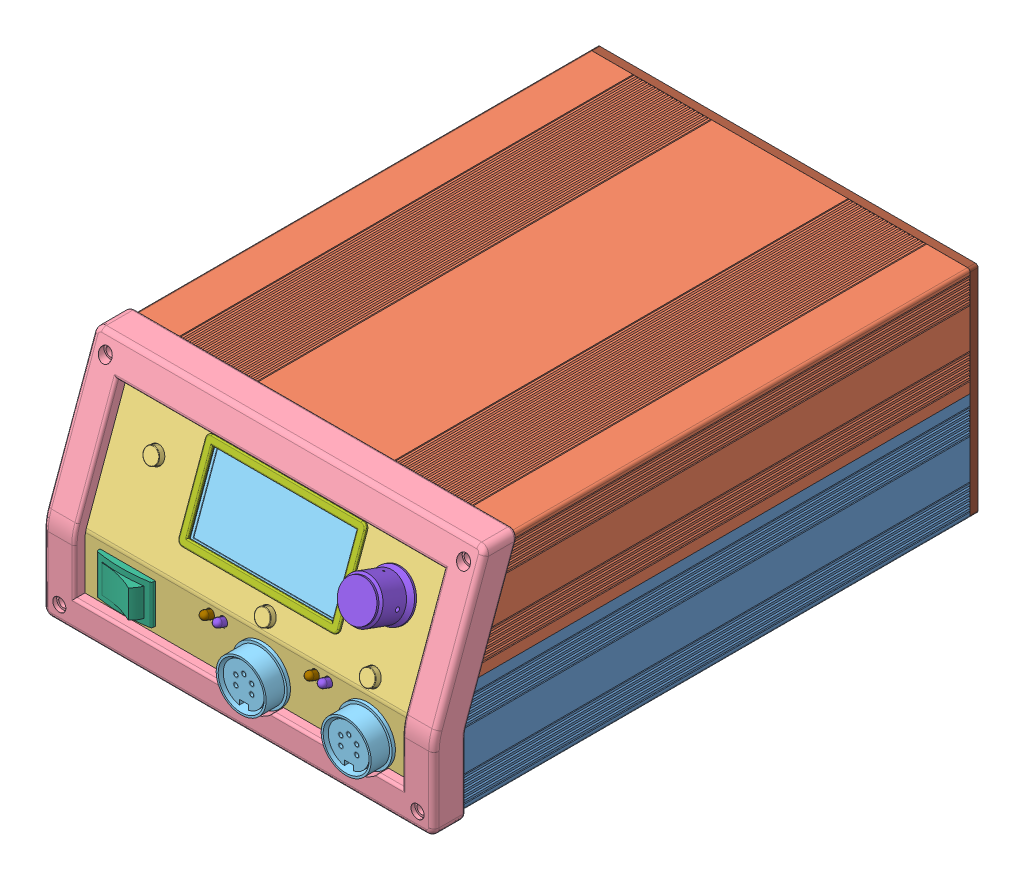
SolidWorks assembly Assembly, configuration Default. Lengths in mm.
Overall size (149 87.32 221.36).
420 component instances, 55 part files, 54 mates.
Components (placement in the parent):
- CaseExtrusion-ModifiedBottom-4: CaseExtrusion-ModifiedBottom [Default] at origin size (145 43.4 200)
- CaseExtrusion-ModifiedTop-7: CaseExtrusion-ModifiedTop [Default] x (-1 0 0) z (0 0 1) size (145 43.1 195.63)
- Front Panel-1: Front Panel [Default] at (72.5 -12 0) x (-1 0 0) z (0 0 -1) size (145 82.88 21.33)
- Front Panel Bezel-2: Front Panel Bezel [Default] at (0 -12 2.3103) x (0 0 1) z (-1 0 0) size (32.14 86.2 149)
- AmphenolSocket-3: AmphenolSocket [Default] at (5 -25.1 3.27) size (21 21 19.77)
- AmphenolSocket-4: AmphenolSocket [Default] at (45 -25.1 3.27) size (21 21 19.77)
- RockerSwitch-1: RockerSwitch [Default] at (-46.5075 -22.4992 2) x (-1 0 0) z (0 0 1) size (21.56 15.01 28.12)
- OledBezel-3: OledBezel [Default] at (0 14.2689 -6.3686) x (-1 0 0) z (0 -0.34202 -0.939693) size (61.1 33.49 3)
- Knob-1: Knob [HEA-A1-1] at (46 17.0964 -6.3335) x (1 0 0) z (0 -0.939693 0.34202) size (17.46 14.29 17.46)
- Transformer Mounting Plate-1: Transformer Mounting Plate [Default] at (0 -33.6 -100) size (115 2 115)
- Triad Magnetics-VPT48-3300-1: Triad Magnetics-VPT48-3300 [Default] at (0 -6.6 -100) x (0.526054 0 -0.850451) z (0.850451 0 0.526054) size (102.88 51 103.1)
- Rear Panel-1: Rear Panel [Default] at (0 0.01 -200) x (0 0 -1) z (1 0 0) size (3 82.2 145)
- IEC_Connector_Fused_Flanges (Schurter 6200)-1: IEC_Connector_Fused_Flanges (Schurter 6200) [Default] at (-44.5 -14.19 -205.5) x (1 0 0) z (0 0 -1) size (44 34 28.25)
- SolderingStation-3: SolderingStation [Default] at (108 -45.1633 3.8854) x (-1 0 0) z (0 -0.34202 -0.939693) size (142.21 62 43.76)
  - SolderingStation.step-1: SolderingStation.step [Default] at origin size (142.21 62 43.76)
    - Board_ss.step-1: Board_ss.step [Default] at origin size (140 62 1.69)
      - Open CASCADE STEP translator 6.8 4.1.1.step-1: Open CASCADE STEP translator 6.8 4.1.1.step [Default] at (0 0 -1.6914) size (140 62 1.69)
    - C17_ss.step-1: C17_ss.step [Default] at origin size (1.25 2 0.78)
      - User_Library-0805_SMD_Capacitor.step-1: User_Library-0805_SMD_Capacitor.step [Default] at (110.8455 64.7701 0) x (0 1 0) z (1 0 0) size (2 0.78 1.25)
    - R45_ss.step-1: R45_ss.step [Default] at origin size (1.7 0.8 0.56)
      - User_Library-RES_1609-0603.step-1: User_Library-RES_1609-0603.step [Default] at (65.2781 57.15 0) x (1 0 0) z (0 -1 0) size (1.7 0.56 0.8)
    - N1_ss.step-1: N1_ss.step [Default] at origin size (9.09 12.8 3.73)
      - nal-clip.step-1: nal-clip.step [Default] at (42.9877 48.2091 -0.8) x (0 0 -1) z (0 -1 0) size (3.73 9.09 12.8)
    - U2_ss.step-1: U2_ss.step [Default] at origin size (6.2 5 1.75)
      - User_Library-SOIC8_JEDEC_MS-012AA.step-1: User_Library-SOIC8_JEDEC_MS-012AA.step [Default] at (80.8676 75.6667 0) x (0 1 0) z (1 0 0) size (5 1.75 6.2)
    - C15_ss.step-1: C15_ss.step [Default] at origin size (1.6 0.8 0.3)
      - User_Library-0603_SMD_Capacitor.step-1: User_Library-0603_SMD_Capacitor.step [Default] at (161.9249 74.0409 0) x (-1 0 0) z (0 1 0) size (1.6 0.3 0.8)
    - C18_ss.step-1: C18_ss.step [Default] at origin size (1.6 0.8 0.3)
      - User_Library-0603_SMD_Capacitor.step-1: User_Library-0603_SMD_Capacitor.step [Default] at (161.9249 75.4379 0) x (-1 0 0) z (0 1 0) size (1.6 0.3 0.8)
    - U10_ss.step-1: U10_ss.step [Default] at origin size (3 2.5 1.1)
      - CircuitWorks-SOT-23.step-1: CircuitWorks-SOT-23.step [Default] at (163.4489 78.7147 0.5) x (-1 0 0) z (0 1 0) size (3 1.1 2.5)
    - U9_ss.step-1: U9_ss.step [Default] at origin size (2.8 2.9 1.45)
      - User_Library-SOT23-5-2.step-1: User_Library-SOT23-5-2.step [Default] at (107.9245 64.4143 0) x (0 -1 0) z (0 0 1) size (2.9 2.8 1.45)
    - C27_ss.step-1: C27_ss.step [Default] at origin size (1.25 2 0.78)
      - User_Library-0805_SMD_Capacitor.step-1: User_Library-0805_SMD_Capacitor.step [Default] at (114.5539 60.8331 0) x (0 1 0) z (1 0 0) size (2 0.78 1.25)
    - C26_ss.step-1: C26_ss.step [Default] at origin size (0.8 1.6 0.3)
      - User_Library-0603_SMD_Capacitor.step-1: User_Library-0603_SMD_Capacitor.step [Default] at (105.0035 64.1605 0) x (0 1 0) z (1 0 0) size (1.6 0.3 0.8)
    - C25_ss.step-1: C25_ss.step [Default] at origin size (1.25 2 0.78)
      - User_Library-0805_SMD_Capacitor.step-1: User_Library-0805_SMD_Capacitor.step [Default] at (109.4741 44.7039 0) x (0 -1 0) z (-1 0 0) size (2 0.78 1.25)
    - C24_ss.step-1: C24_ss.step [Default] at origin size (1.25 2 0.78)
      - User_Library-0805_SMD_Capacitor.step-1: User_Library-0805_SMD_Capacitor.step [Default] at (69.5961 44.4499 0) x (0 -1 0) z (-1 0 0) size (2 0.78 1.25)
    - D13_ss.step-1: D13_ss.step [Default] at origin size (2.7 1.25 1.1)
      - User_Library-SOD2513X11.step-1: User_Library-SOD2513X11.step [Default] at (167.7671 78.5115 0) x (1 0 0) z (0 0 1) size (2.7 1.25 1.1)
    - C22_ss.step-1: C22_ss.step [Default] at origin size (2 1.25 0.78)
      - User_Library-0805_SMD_Capacitor.step-1: User_Library-0805_SMD_Capacitor.step [Default] at (105.3871 57.6581 0) x (1 0 0) z (0 -1 0) size (2 0.78 1.25)
    - C23_ss.step-1: C23_ss.step [Default] at origin size (2 1.25 0.78)
      - User_Library-0805_SMD_Capacitor.step-1: User_Library-0805_SMD_Capacitor.step [Default] at (111.2291 57.6581 0) x (1 0 0) z (0 -1 0) size (2 0.78 1.25)
    - C21_ss.step-1: C21_ss.step [Default] at origin size (1.6 0.8 0.3)
      - User_Library-0603_SMD_Capacitor.step-1: User_Library-0603_SMD_Capacitor.step [Default] at (102.3367 85.0901 0) x (1 0 0) z (0 -1 0) size (1.6 0.3 0.8)
    - SP6_ss.step-1: SP6_ss.step [Default] at origin size (6 6 6)
      - 6mmSpacer.step-1: 6mmSpacer.step [Default] at (46.8629 36.8301 -1.6914) x (-1 0 0) z (0 -1 0) size (6 6 6)
    - SP5_ss.step-1: SP5_ss.step [Default] at origin size (6 6 6)
      - 6mmSpacer.step-1: 6mmSpacer.step [Default] at (169.9259 46.8631 -1.6914) x (-1 0 0) z (0 -1 0) size (6 6 6)
    - D2_ss.step-1: D2_ss.step [Default] at origin size (2.7 1.25 1.1)
      - User_Library-SOD2513X11.step-1: User_Library-SOD2513X11.step [Default] at (125.2719 47.6779 0) x (-1 0 0) z (0 0 1) size (2.7 1.25 1.1)
    - U1_ss.step-1: U1_ss.step [Default] at origin size (9.94 6.54 2.42)
      - User_Library-DPAK-1.step-1: User_Library-DPAK-1.step [Default] at (105.596 76.2 1.15) x (0 -1 0) z (-1 0 0) size (6.54 2.42 9.94)
    - C20_ss.step-1: C20_ss.step [Default] at origin size (0.8 1.6 0.3)
      - User_Library-0603_SMD_Capacitor.step-1: User_Library-0603_SMD_Capacitor.step [Default] at (132.4355 61.1887 0) x (0 1 0) z (1 0 0) size (1.6 0.3 0.8)
    - C7_ss.step-1: C7_ss.step [Default] at origin size (0.8 1.6 0.3)
      - User_Library-0603_SMD_Capacitor.step-1: User_Library-0603_SMD_Capacitor.step [Default] at (92.3797 61.1631 0) x (0 1 0) z (1 0 0) size (1.6 0.3 0.8)
    - P1_ss.step-1: P1_ss.step [Default] at origin size (10.62 6.5 13.4)
      - c-282834-4-c-3d.step-1: c-282834-4-c-3d.step [Default] at (138.4201 36.0681 10) size (10.62 6.5 13.4)
    - R25_ss.step-1: R25_ss.step [Default] at origin size (1.65 16.48 27.41)
      - OAR3.step-1: OAR3.step [Default] at (70.9931 46.1009 -3.2) x (0 -1 0) z (-1 0 0) size (16.48 27.41 1.65)
    - R26_ss.step-1: R26_ss.step [Default] at origin size (1.65 16.48 27.41)
      - OAR3.step-1: OAR3.step [Default] at (111.1505 46.1009 -3.2) x (0 -1 0) z (-1 0 0) size (16.48 27.41 1.65)
    - R19_ss.step-1: R19_ss.step [Default] at origin size (0.8 1.7 0.56)
      - User_Library-RES_1609-0603.step-1: User_Library-RES_1609-0603.step [Default] at (154.101 48.0431 0) x (0 1 0) z (1 0 0) size (1.7 0.56 0.8)
    - R20_ss.step-1: R20_ss.step [Default] at origin size (0.8 1.7 0.56)
      - User_Library-RES_1609-0603.step-1: User_Library-RES_1609-0603.step [Default] at (156.1329 48.0431 0) x (0 1 0) z (1 0 0) size (1.7 0.56 0.8)
    - R27_ss.step-1: R27_ss.step [Default] at origin size (0.8 1.7 0.56)
      - User_Library-RES_1609-0603.step-1: User_Library-RES_1609-0603.step [Default] at (154.101 40.5501 0) x (0 1 0) z (1 0 0) size (1.7 0.56 0.8)
    - R28_ss.step-1: R28_ss.step [Default] at origin size (0.8 1.7 0.56)
      - User_Library-RES_1609-0603.step-1: User_Library-RES_1609-0603.step [Default] at (156.1329 40.5501 0) x (0 1 0) z (1 0 0) size (1.7 0.56 0.8)
    - D11_ss.step-1: D11_ss.step [Default] at origin size (3.5 3.8 10)
      - Red-LED_3MM.step-1: Red-LED_3MM.step [Default] at (77.9999 28.5001 -5.6914) x (0 1 0) z (0 0 -1) size (3.8 3.5 10)
    - D9_ss.step-1: D9_ss.step [Default] at origin size (3.5 3.8 10)
      - Red-LED_3MM.step-1: Red-LED_3MM.step [Default] at (117.9999 28.5001 -5.6914) x (0 1 0) z (0 0 -1) size (3.8 3.5 10)
    - D10_ss.step-1: D10_ss.step [Default] at origin size (3.5 3.8 10)
      - Green-LED_3MM.step-1: Green-LED_3MM.step [Default] at (122.9999 28.5001 -5.6914) x (0 1 0) z (0 0 -1) size (3.8 3.5 10)
    - D12_ss.step-1: D12_ss.step [Default] at origin size (3.5 3.8 10)
      - Green-LED_3MM.step-1: Green-LED_3MM.step [Default] at (82.9999 28.5001 -5.6914) x (0 1 0) z (0 0 -1) size (3.8 3.5 10)
    - S2_ss.step-1: S2_ss.step [Default] at origin size (7.7 6 10.2)
      - User_Library-b3w1050.step-1: User_Library-b3w1050.step [Default] at (63 36.9999 -1.6914) x (1 0 0) z (0 1 0) size (3.5 1.6 3.5)
      - User_Library-b3w1050.step-2: User_Library-b3w1050.step [Default] at (63 36.9999 -1.6914) x (1 0 0) z (0 1 0) size (3.5 1.6 3.5)
      - User_Library-b3w1050-0.step-1: User_Library-b3w1050-0.step [Default] at (63 36.9999 -1.6914) x (1 0 0) z (0 1 0) size (3.5 1.6 3.5)
      - User_Library-b3w1050-1.step-1: User_Library-b3w1050-1.step [Default] at (63 36.9999 -1.6914) x (1 0 0) z (0 1 0) size (7.7 10.2 6)
      - User_Library-b3w1050-1.step-2: User_Library-b3w1050-1.step [Default] at (63 36.9999 -1.6914) x (1 0 0) z (0 1 0) size (7.7 10.2 6)
      - User_Library-b3w1050-2.step-1: User_Library-b3w1050-2.step [Default] at (63 36.9999 -1.6914) x (1 0 0) z (0 1 0) size (7.7 10.2 6)
    - S1_ss.step-1: S1_ss.step [Default] at origin size (7.7 6 10.2)
      - User_Library-b3w1050.step-1: User_Library-b3w1050.step [Default] at (154 62.0001 -1.6914) x (-1 0 0) z (0 -1 0) size (3.5 1.6 3.5)
      - User_Library-b3w1050.step-2: User_Library-b3w1050.step [Default] at (154 62.0001 -1.6914) x (-1 0 0) z (0 -1 0) size (3.5 1.6 3.5)
      - User_Library-b3w1050-0.step-1: User_Library-b3w1050-0.step [Default] at (154 62.0001 -1.6914) x (-1 0 0) z (0 -1 0) size (3.5 1.6 3.5)
      - User_Library-b3w1050-1.step-1: User_Library-b3w1050-1.step [Default] at (154 62.0001 -1.6914) x (-1 0 0) z (0 -1 0) size (7.7 10.2 6)
      - User_Library-b3w1050-1.step-2: User_Library-b3w1050-1.step [Default] at (154 62.0001 -1.6914) x (-1 0 0) z (0 -1 0) size (7.7 10.2 6)
      - User_Library-b3w1050-2.step-1: User_Library-b3w1050-2.step [Default] at (154 62.0001 -1.6914) x (-1 0 0) z (0 -1 0) size (7.7 10.2 6)
    - S3_ss.step-1: S3_ss.step [Default] at origin size (7.7 6 10.2)
      - User_Library-b3w1050.step-1: User_Library-b3w1050.step [Default] at (103 36.9999 -1.6914) x (1 0 0) z (0 1 0) size (3.5 1.6 3.5)
      - User_Library-b3w1050.step-2: User_Library-b3w1050.step [Default] at (103 36.9999 -1.6914) x (1 0 0) z (0 1 0) size (3.5 1.6 3.5)
      - User_Library-b3w1050-0.step-1: User_Library-b3w1050-0.step [Default] at (103 36.9999 -1.6914) x (1 0 0) z (0 1 0) size (3.5 1.6 3.5)
      - User_Library-b3w1050-1.step-1: User_Library-b3w1050-1.step [Default] at (103 36.9999 -1.6914) x (1 0 0) z (0 1 0) size (7.7 10.2 6)
      - User_Library-b3w1050-1.step-2: User_Library-b3w1050-1.step [Default] at (103 36.9999 -1.6914) x (1 0 0) z (0 1 0) size (7.7 10.2 6)
      - User_Library-b3w1050-2.step-1: User_Library-b3w1050-2.step [Default] at (103 36.9999 -1.6914) x (1 0 0) z (0 1 0) size (7.7 10.2 6)
    - U5_ss.step-1: U5_ss.step [Default] at origin size (9 9 1.6)
      - User_Library-LQFP48_Grid_0.5.step-1: User_Library-LQFP48_Grid_0.5.step [Default] at (153.5238 71.918 0) x (0 1 0) z (1 0 0) size (9 1.6 9)
        - User_Library-LQFP48_Grid_0.5_LQFP48_Koerper_2.step-1: User_Library-LQFP48_Grid_0.5_LQFP48_Koerper_2.step [Default] at origin size (7 1.45 7)
        - User_Library-LQFP48_Grid_0.5_LQFP_PIN_2.step-1: User_Library-LQFP48_Grid_0.5_LQFP_PIN_2.step [Default] at (-2.75 0 4.5) size (0.27 0.97 1.5)
        - User_Library-LQFP48_Grid_0.5_LQFP_PIN_2.step-2: User_Library-LQFP48_Grid_0.5_LQFP_PIN_2.step [Default] at (-2.25 0 4.5) size (0.27 0.97 1.5)
        - User_Library-LQFP48_Grid_0.5_LQFP_PIN_2.step-3: User_Library-LQFP48_Grid_0.5_LQFP_PIN_2.step [Default] at (-1.75 0 4.5) size (0.27 0.97 1.5)
        - User_Library-LQFP48_Grid_0.5_LQFP_PIN_2.step-4: User_Library-LQFP48_Grid_0.5_LQFP_PIN_2.step [Default] at (-1.25 0 4.5) size (0.27 0.97 1.5)
        - User_Library-LQFP48_Grid_0.5_LQFP_PIN_2.step-5: User_Library-LQFP48_Grid_0.5_LQFP_PIN_2.step [Default] at (-0.75 0 4.5) size (0.27 0.97 1.5)
        - User_Library-LQFP48_Grid_0.5_LQFP_PIN_2.step-6: User_Library-LQFP48_Grid_0.5_LQFP_PIN_2.step [Default] at (-0.25 0 4.5) size (0.27 0.97 1.5)
        - User_Library-LQFP48_Grid_0.5_LQFP_PIN_2.step-7: User_Library-LQFP48_Grid_0.5_LQFP_PIN_2.step [Default] at (0.25 0 4.5) size (0.27 0.97 1.5)
        - User_Library-LQFP48_Grid_0.5_LQFP_PIN_2.step-8: User_Library-LQFP48_Grid_0.5_LQFP_PIN_2.step [Default] at (0.75 0 4.5) size (0.27 0.97 1.5)
        - User_Library-LQFP48_Grid_0.5_LQFP_PIN_2.step-9: User_Library-LQFP48_Grid_0.5_LQFP_PIN_2.step [Default] at (1.25 0 4.5) size (0.27 0.97 1.5)
        - User_Library-LQFP48_Grid_0.5_LQFP_PIN_2.step-10: User_Library-LQFP48_Grid_0.5_LQFP_PIN_2.step [Default] at (1.75 0 4.5) size (0.27 0.97 1.5)
        - User_Library-LQFP48_Grid_0.5_LQFP_PIN_2.step-11: User_Library-LQFP48_Grid_0.5_LQFP_PIN_2.step [Default] at (2.25 0 4.5) size (0.27 0.97 1.5)
        - User_Library-LQFP48_Grid_0.5_LQFP_PIN_2.step-12: User_Library-LQFP48_Grid_0.5_LQFP_PIN_2.step [Default] at (2.75 0 4.5) size (0.27 0.97 1.5)
        - User_Library-LQFP48_Grid_0.5_LQFP_PIN_2.step-13: User_Library-LQFP48_Grid_0.5_LQFP_PIN_2.step [Default] at (4.5 0 2.75) x (0 0 -1) z (1 0 0) size (0.27 0.97 1.5)
        - User_Library-LQFP48_Grid_0.5_LQFP_PIN_2.step-14: User_Library-LQFP48_Grid_0.5_LQFP_PIN_2.step [Default] at (4.5 0 2.25) x (0 0 -1) z (1 0 0) size (0.27 0.97 1.5)
        - User_Library-LQFP48_Grid_0.5_LQFP_PIN_2.step-15: User_Library-LQFP48_Grid_0.5_LQFP_PIN_2.step [Default] at (4.5 0 1.75) x (0 0 -1) z (1 0 0) size (0.27 0.97 1.5)
        - User_Library-LQFP48_Grid_0.5_LQFP_PIN_2.step-16: User_Library-LQFP48_Grid_0.5_LQFP_PIN_2.step [Default] at (4.5 0 1.25) x (0 0 -1) z (1 0 0) size (0.27 0.97 1.5)
        - User_Library-LQFP48_Grid_0.5_LQFP_PIN_2.step-17: User_Library-LQFP48_Grid_0.5_LQFP_PIN_2.step [Default] at (4.5 0 0.75) x (0 0 -1) z (1 0 0) size (0.27 0.97 1.5)
        - User_Library-LQFP48_Grid_0.5_LQFP_PIN_2.step-18: User_Library-LQFP48_Grid_0.5_LQFP_PIN_2.step [Default] at (4.5 0 0.25) x (0 0 -1) z (1 0 0) size (0.27 0.97 1.5)
        - User_Library-LQFP48_Grid_0.5_LQFP_PIN_2.step-19: User_Library-LQFP48_Grid_0.5_LQFP_PIN_2.step [Default] at (4.5 0 -0.25) x (0 0 -1) z (1 0 0) size (0.27 0.97 1.5)
        - User_Library-LQFP48_Grid_0.5_LQFP_PIN_2.step-20: User_Library-LQFP48_Grid_0.5_LQFP_PIN_2.step [Default] at (4.5 0 -0.75) x (0 0 -1) z (1 0 0) size (0.27 0.97 1.5)
        - User_Library-LQFP48_Grid_0.5_LQFP_PIN_2.step-21: User_Library-LQFP48_Grid_0.5_LQFP_PIN_2.step [Default] at (4.5 0 -1.25) x (0 0 -1) z (1 0 0) size (0.27 0.97 1.5)
        - User_Library-LQFP48_Grid_0.5_LQFP_PIN_2.step-22: User_Library-LQFP48_Grid_0.5_LQFP_PIN_2.step [Default] at (4.5 0 -1.75) x (0 0 -1) z (1 0 0) size (0.27 0.97 1.5)
        - User_Library-LQFP48_Grid_0.5_LQFP_PIN_2.step-23: User_Library-LQFP48_Grid_0.5_LQFP_PIN_2.step [Default] at (4.5 0 -2.25) x (0 0 -1) z (1 0 0) size (0.27 0.97 1.5)
        - User_Library-LQFP48_Grid_0.5_LQFP_PIN_2.step-24: User_Library-LQFP48_Grid_0.5_LQFP_PIN_2.step [Default] at (4.5 0 -2.75) x (0 0 -1) z (1 0 0) size (0.27 0.97 1.5)
        - User_Library-LQFP48_Grid_0.5_LQFP_PIN_2.step-25: User_Library-LQFP48_Grid_0.5_LQFP_PIN_2.step [Default] at (2.75 0 -4.5) x (-1 0 0) z (0 0 -1) size (0.27 0.97 1.5)
        - User_Library-LQFP48_Grid_0.5_LQFP_PIN_2.step-26: User_Library-LQFP48_Grid_0.5_LQFP_PIN_2.step [Default] at (2.25 0 -4.5) x (-1 0 0) z (0 0 -1) size (0.27 0.97 1.5)
        - User_Library-LQFP48_Grid_0.5_LQFP_PIN_2.step-27: User_Library-LQFP48_Grid_0.5_LQFP_PIN_2.step [Default] at (1.75 0 -4.5) x (-1 0 0) z (0 0 -1) size (0.27 0.97 1.5)
        - User_Library-LQFP48_Grid_0.5_LQFP_PIN_2.step-28: User_Library-LQFP48_Grid_0.5_LQFP_PIN_2.step [Default] at (1.25 0 -4.5) x (-1 0 0) z (0 0 -1) size (0.27 0.97 1.5)
        - User_Library-LQFP48_Grid_0.5_LQFP_PIN_2.step-29: User_Library-LQFP48_Grid_0.5_LQFP_PIN_2.step [Default] at (0.75 0 -4.5) x (-1 0 0) z (0 0 -1) size (0.27 0.97 1.5)
        - User_Library-LQFP48_Grid_0.5_LQFP_PIN_2.step-30: User_Library-LQFP48_Grid_0.5_LQFP_PIN_2.step [Default] at (0.25 0 -4.5) x (-1 0 0) z (0 0 -1) size (0.27 0.97 1.5)
        - User_Library-LQFP48_Grid_0.5_LQFP_PIN_2.step-31: User_Library-LQFP48_Grid_0.5_LQFP_PIN_2.step [Default] at (-0.25 0 -4.5) x (-1 0 0) z (0 0 -1) size (0.27 0.97 1.5)
        - User_Library-LQFP48_Grid_0.5_LQFP_PIN_2.step-32: User_Library-LQFP48_Grid_0.5_LQFP_PIN_2.step [Default] at (-0.75 0 -4.5) x (-1 0 0) z (0 0 -1) size (0.27 0.97 1.5)
        - User_Library-LQFP48_Grid_0.5_LQFP_PIN_2.step-33: User_Library-LQFP48_Grid_0.5_LQFP_PIN_2.step [Default] at (-1.25 0 -4.5) x (-1 0 0) z (0 0 -1) size (0.27 0.97 1.5)
        - User_Library-LQFP48_Grid_0.5_LQFP_PIN_2.step-34: User_Library-LQFP48_Grid_0.5_LQFP_PIN_2.step [Default] at (-1.75 0 -4.5) x (-1 0 0) z (0 0 -1) size (0.27 0.97 1.5)
        - User_Library-LQFP48_Grid_0.5_LQFP_PIN_2.step-35: User_Library-LQFP48_Grid_0.5_LQFP_PIN_2.step [Default] at (-2.25 0 -4.5) x (-1 0 0) z (0 0 -1) size (0.27 0.97 1.5)
        - User_Library-LQFP48_Grid_0.5_LQFP_PIN_2.step-36: User_Library-LQFP48_Grid_0.5_LQFP_PIN_2.step [Default] at (-2.75 0 -4.5) x (-1 0 0) z (0 0 -1) size (0.27 0.97 1.5)
        - User_Library-LQFP48_Grid_0.5_LQFP_PIN_2.step-37: User_Library-LQFP48_Grid_0.5_LQFP_PIN_2.step [Default] at (-4.5 0 -2.75) x (0 0 1) z (-1 0 0) size (0.27 0.97 1.5)
        - User_Library-LQFP48_Grid_0.5_LQFP_PIN_2.step-38: User_Library-LQFP48_Grid_0.5_LQFP_PIN_2.step [Default] at (-4.5 0 -2.25) x (0 0 1) z (-1 0 0) size (0.27 0.97 1.5)
        - User_Library-LQFP48_Grid_0.5_LQFP_PIN_2.step-39: User_Library-LQFP48_Grid_0.5_LQFP_PIN_2.step [Default] at (-4.5 0 -1.75) x (0 0 1) z (-1 0 0) size (0.27 0.97 1.5)
        - User_Library-LQFP48_Grid_0.5_LQFP_PIN_2.step-40: User_Library-LQFP48_Grid_0.5_LQFP_PIN_2.step [Default] at (-4.5 0 -1.25) x (0 0 1) z (-1 0 0) size (0.27 0.97 1.5)
        - User_Library-LQFP48_Grid_0.5_LQFP_PIN_2.step-41: User_Library-LQFP48_Grid_0.5_LQFP_PIN_2.step [Default] at (-4.5 0 -0.75) x (0 0 1) z (-1 0 0) size (0.27 0.97 1.5)
        - User_Library-LQFP48_Grid_0.5_LQFP_PIN_2.step-42: User_Library-LQFP48_Grid_0.5_LQFP_PIN_2.step [Default] at (-4.5 0 -0.25) x (0 0 1) z (-1 0 0) size (0.27 0.97 1.5)
        - User_Library-LQFP48_Grid_0.5_LQFP_PIN_2.step-43: User_Library-LQFP48_Grid_0.5_LQFP_PIN_2.step [Default] at (-4.5 0 0.25) x (0 0 1) z (-1 0 0) size (0.27 0.97 1.5)
        - User_Library-LQFP48_Grid_0.5_LQFP_PIN_2.step-44: User_Library-LQFP48_Grid_0.5_LQFP_PIN_2.step [Default] at (-4.5 0 0.75) x (0 0 1) z (-1 0 0) size (0.27 0.97 1.5)
        - User_Library-LQFP48_Grid_0.5_LQFP_PIN_2.step-45: User_Library-LQFP48_Grid_0.5_LQFP_PIN_2.step [Default] at (-4.5 0 1.25) x (0 0 1) z (-1 0 0) size (0.27 0.97 1.5)
        - User_Library-LQFP48_Grid_0.5_LQFP_PIN_2.step-46: User_Library-LQFP48_Grid_0.5_LQFP_PIN_2.step [Default] at (-4.5 0 1.75) x (0 0 1) z (-1 0 0) size (0.27 0.97 1.5)
        - User_Library-LQFP48_Grid_0.5_LQFP_PIN_2.step-47: User_Library-LQFP48_Grid_0.5_LQFP_PIN_2.step [Default] at (-4.5 0 2.25) x (0 0 1) z (-1 0 0) size (0.27 0.97 1.5)
        - User_Library-LQFP48_Grid_0.5_LQFP_PIN_2.step-48: User_Library-LQFP48_Grid_0.5_LQFP_PIN_2.step [Default] at (-4.5 0 2.75) x (0 0 1) z (-1 0 0) size (0.27 0.97 1.5)
    - C12_ss.step-1: C12_ss.step [Default] at origin size (1.6 0.8 0.3)
      - User_Library-0603_SMD_Capacitor.step-1: User_Library-0603_SMD_Capacitor.step [Default] at (167.9195 75.9461 0) x (1 0 0) z (0 -1 0) size (1.6 0.3 0.8)
    - C13_ss.step-1: C13_ss.step [Default] at origin size (1.6 0.8 0.3)
      - User_Library-0603_SMD_Capacitor.step-1: User_Library-0603_SMD_Capacitor.step [Default] at (161.9249 72.1359 0) x (-1 0 0) z (0 1 0) size (1.6 0.3 0.8)
    - C14_ss.step-1: C14_ss.step [Default] at origin size (1.6 0.8 0.3)
      - User_Library-0603_SMD_Capacitor.step-1: User_Library-0603_SMD_Capacitor.step [Default] at (150.8761 78.6131 0) x (1 0 0) z (0 -1 0) size (1.6 0.3 0.8)
    - C16_ss.step-1: C16_ss.step [Default] at origin size (1.6 0.8 0.3)
      - User_Library-0603_SMD_Capacitor.step-1: User_Library-0603_SMD_Capacitor.step [Default] at (160.3239 66.9819 0) x (-1 0 0) z (0 1 0) size (1.6 0.3 0.8)
    - P6_ss.step-1: P6_ss.step [Default] at origin size (6.35 3.4 6.8)
      - SWD2x5.step-1: SWD2x5.step [Default] at (153.0859 83.8493 0) x (1 0 0) z (0 -1 0) size (6.35 6.8 3.4)
    - R38_ss.step-1: R38_ss.step [Default] at origin size (1.7 0.8 0.56)
      - User_Library-RES_1609-0603.step-1: User_Library-RES_1609-0603.step [Default] at (159.9431 62.537 0) x (1 0 0) z (0 -1 0) size (1.7 0.56 0.8)
    - R37_ss.step-1: R37_ss.step [Default] at origin size (1.7 0.8 0.56)
      - User_Library-RES_1609-0603.step-1: User_Library-RES_1609-0603.step [Default] at (159.9431 63.807 0) x (1 0 0) z (0 -1 0) size (1.7 0.56 0.8)
    - R40_ss.step-1: R40_ss.step [Default] at origin size (1.7 0.8 0.56)
      - User_Library-RES_1609-0603.step-1: User_Library-RES_1609-0603.step [Default] at (159.9431 61.267 0) x (1 0 0) z (0 -1 0) size (1.7 0.56 0.8)
    - R39_ss.step-1: R39_ss.step [Default] at origin size (1.7 0.8 0.56)
      - User_Library-RES_1609-0603.step-1: User_Library-RES_1609-0603.step [Default] at (172.3891 66.7281 0) x (1 0 0) z (0 -1 0) size (1.7 0.56 0.8)
    - R41_ss.step-1: R41_ss.step [Default] at origin size (1.7 0.8 0.56)
      - User_Library-RES_1609-0603.step-1: User_Library-RES_1609-0603.step [Default] at (172.3889 79.936 0) x (-1 0 0) z (0 1 0) size (1.7 0.56 0.8)
    - R42_ss.step-1: R42_ss.step [Default] at origin size (1.7 0.8 0.56)
      - User_Library-RES_1609-0603.step-1: User_Library-RES_1609-0603.step [Default] at (161.8479 70.5379 0) x (-1 0 0) z (0 1 0) size (1.7 0.56 0.8)
    - R43_ss.step-1: R43_ss.step [Default] at origin size (1.7 0.8 0.56)
      - User_Library-RES_1609-0603.step-1: User_Library-RES_1609-0603.step [Default] at (161.8479 69.268 0) x (-1 0 0) z (0 1 0) size (1.7 0.56 0.8)
    - R50_ss.step-1: R50_ss.step [Default] at origin size (1.7 0.8 0.56)
      - User_Library-RES_1609-0603.step-1: User_Library-RES_1609-0603.step [Default] at (77.5201 31.406 0) x (1 0 0) z (0 -1 0) size (1.7 0.56 0.8)
    - R47_ss.step-1: R47_ss.step [Default] at origin size (1.7 0.8 0.56)
      - User_Library-RES_1609-0603.step-1: User_Library-RES_1609-0603.step [Default] at (117.6519 31.422 0) x (-1 0 0) z (0 1 0) size (1.7 0.56 0.8)
    - R49_ss.step-1: R49_ss.step [Default] at origin size (1.7 0.8 0.56)
      - User_Library-RES_1609-0603.step-1: User_Library-RES_1609-0603.step [Default] at (122.7321 31.422 0) x (1 0 0) z (0 -1 0) size (1.7 0.56 0.8)
    - R52_ss.step-1: R52_ss.step [Default] at origin size (1.7 0.8 0.56)
      - User_Library-RES_1609-0603.step-1: User_Library-RES_1609-0603.step [Default] at (82.6001 31.406 0) x (1 0 0) z (0 -1 0) size (1.7 0.56 0.8)
    - R51_ss.step-1: R51_ss.step [Default] at origin size (1.7 0.8 0.56)
      - User_Library-RES_1609-0603.step-1: User_Library-RES_1609-0603.step [Default] at (71.3999 62 0) x (-1 0 0) z (0 1 0) size (1.7 0.56 0.8)
    - R53_ss.step-1: R53_ss.step [Default] at origin size (1.7 0.8 0.56)
      - User_Library-RES_1609-0603.step-1: User_Library-RES_1609-0603.step [Default] at (71.3999 64.5 0) x (-1 0 0) z (0 1 0) size (1.7 0.56 0.8)
    - Y1_ss.step-1: Y1_ss.step [Default] at origin size (2.5 3.2 0.7)
      - EPSON-FA-238.step-1: EPSON-FA-238.step [Default] at (146.624 78.2189 0) x (0 1 0) z (1 0 0) size (3.2 0.7 2.5)
    - Z1_ss.step-1: Z1_ss.step [Default] at origin size (2.84 2.9 1.28)
      - SOT-23-6_(SOT457,SC-74).step-1: SOT-23-6_(SOT457,SC-74).step [Default] at (167.3089 71.8081 0.1) x (1 0 0) z (0 -1 0) size (2.84 1.28 2.9)
    - Q9_ss.step-1: Q9_ss.step [Default] at origin size (5 6.2 1.75)
      - User_Library-SOIC8_JEDEC_MS-012AA.step-1: User_Library-SOIC8_JEDEC_MS-012AA.step [Default] at (160.7051 38.7721 0) x (1 0 0) z (0 -1 0) size (5 1.75 6.2)
    - Q10_ss.step-1: Q10_ss.step [Default] at origin size (5 6.2 1.75)
      - User_Library-SOIC8_JEDEC_MS-012AA.step-1: User_Library-SOIC8_JEDEC_MS-012AA.step [Default] at (149.5291 38.7721 0) x (1 0 0) z (0 -1 0) size (5 1.75 6.2)
    - Q8_ss.step-1: Q8_ss.step [Default] at origin size (5 6.2 1.75)
      - User_Library-SOIC8_JEDEC_MS-012AA.step-1: User_Library-SOIC8_JEDEC_MS-012AA.step [Default] at (160.7049 49.9479 0) x (-1 0 0) z (0 1 0) size (5 1.75 6.2)
    - Q7_ss.step-1: Q7_ss.step [Default] at origin size (5 6.2 1.75)
      - User_Library-SOIC8_JEDEC_MS-012AA.step-1: User_Library-SOIC8_JEDEC_MS-012AA.step [Default] at (149.5289 49.9479 0) x (-1 0 0) z (0 1 0) size (5 1.75 6.2)
    - D6_ss.step-1: D6_ss.step [Default] at origin size (3 2.5 1.1)
      - CircuitWorks-SOT-23.step-1: CircuitWorks-SOT-23.step [Default] at (155.1171 37.2479 0.5) x (1 0 0) z (0 -1 0) size (3 1.1 2.5)
    - D5_ss.step-1: D5_ss.step [Default] at origin size (3 2.5 1.1)
      - CircuitWorks-SOT-23.step-1: CircuitWorks-SOT-23.step [Default] at (155.1169 51.472 0.5) x (-1 0 0) z (0 1 0) size (3 1.1 2.5)
    - USB1_ss.step-1: USB1_ss.step [Default] at origin size (9.17 9.03 5.56)
      - USB4085-03-A_revA.step-1: USB4085-03-A_revA.step [Default] at (179.7088 73.2001 0) x (0 1 0) z (1 0 0) size (9.03 5.56 9.17)
        - shell_1___.step-1: shell_1___.step [Default] at origin size (8.96 5.56 9.15)
        - housing_1___.step-1: housing_1___.step [Default] at (0 3.15 0) x (1 0 0) z (0 1 0) size (9.03 9.07 4.75)
    - SC2_ss.step-1: SC2_ss.step [Default] at origin size (6 6 5.5)
      - Switch-Cap_-_b32-2000.step-1: Switch-Cap_-_b32-2000.step [Default] at (62.9999 37.0001 -6.1914) x (-1 0 0) z (0 -1 0) size (6 5.5 6)
    - SC3_ss.step-1: SC3_ss.step [Default] at origin size (6 6 5.5)
      - Switch-Cap_-_b32-2000.step-1: Switch-Cap_-_b32-2000.step [Default] at (102.9999 37.0001 -6.1914) x (-1 0 0) z (0 -1 0) size (6 5.5 6)
    - SC1_ss.step-1: SC1_ss.step [Default] at origin size (6 6 5.5)
      - Switch-Cap_-_b32-2000.step-1: Switch-Cap_-_b32-2000.step [Default] at (153.9999 62.0001 -6.1914) x (-1 0 0) z (0 -1 0) size (6 5.5 6)
    - E1_ss.step-1: E1_ss.step [Default] at origin size (15.01 15 22.55)
      - RotaryEncoder.step-1: RotaryEncoder.step [Default] at (62.0001 61.9999 -7.8414) x (1 0 0) z (0 -1 0) size (15.01 22.55 15)
    - OLED1_ss.step-1: OLED1_ss.step [Default] at origin size (72 43 12.5)
      - OLED_128x64_2-42inch.step-1: OLED_128x64_2-42inch.step [Default] at (108.0081 61.9493 -4.1914) x (1 0 0) z (0 1 0) size (72 12.5 43)
    - P2_ss.step-1: P2_ss.step [Default] at origin size (10.15 8.77 13.09)
      - 430450412.step-1: 430450412.step [Default] at (63.0001 45.397 5) x (1 0 0) z (0 0 1) size (10.15 8.77 13.09)
    - P3_ss.step-1: P3_ss.step [Default] at origin size (10.15 8.77 13.09)
      - 430450412.step-1: 430450412.step [Default] at (103.0001 45.397 5) x (1 0 0) z (0 0 1) size (10.15 8.77 13.09)
    - Q1_ss.step-1: Q1_ss.step [Default] at origin size (6.2 5 1.75)
      - User_Library-SOIC8_JEDEC_MS-012AA.step-1: User_Library-SOIC8_JEDEC_MS-012AA.step [Default] at (83.1079 43.4711 0) x (0 1 0) z (1 0 0) size (5 1.75 6.2)
    - R5_ss.step-1: R5_ss.step [Default] at origin size (1.7 0.8 0.56)
      - User_Library-RES_1609-0603.step-1: User_Library-RES_1609-0603.step [Default] at (84.1241 49.456 0) x (1 0 0) z (0 -1 0) size (1.7 0.56 0.8)
    - SP1_ss.step-1: SP1_ss.step [Default] at origin size (6 6 6)
      - 6mmSpacer.step-1: 6mmSpacer.step [Default] at (57.9999 84.0001 -1.6914) x (-1 0 0) z (0 -1 0) size (6 6 6)
    - SP2_ss.step-1: SP2_ss.step [Default] at origin size (6 6 6)
      - 6mmSpacer.step-1: 6mmSpacer.step [Default] at (41.9999 62.0001 -1.6914) x (-1 0 0) z (0 -1 0) size (6 6 6)
    - SP3_ss.step-1: SP3_ss.step [Default] at origin size (6 6 6)
      - 6mmSpacer.step-1: 6mmSpacer.step [Default] at (173.9999 62.0001 -1.6914) x (-1 0 0) z (0 -1 0) size (6 6 6)
    - SP4_ss.step-1: SP4_ss.step [Default] at origin size (6 6 6)
      - 6mmSpacer.step-1: 6mmSpacer.step [Default] at (157.9999 84.0001 -1.6914) x (-1 0 0) z (0 -1 0) size (6 6 6)
    - BR1_ss.step-1: BR1_ss.step [Default] at origin size (7 4.7 2.4)
      - FullWaveRectifier.step-1: FullWaveRectifier.step [Default] at (81.5339 83.5661 0.1) x (0 1 0) z (1 0 0) size (4.7 2.4 7)
    - C2_ss.step-1: C2_ss.step [Default] at origin size (1.25 2 0.78)
      - User_Library-0805_SMD_Capacitor.step-1: User_Library-0805_SMD_Capacitor.step [Default] at (112.2681 76.7079 0) x (0 -1 0) z (-1 0 0) size (2 0.78 1.25)
    - J2_ss.step-1: J2_ss.step [Default] at origin size (9.9 6.1 10.4)
      - User_Library-XH-A-3.step-1: User_Library-XH-A-3.step [Default] at (96.3901 87.3751 7) x (-1 0 0) z (0 0 1) size (9.9 6.1 10.4)
    - R1_ss.step-1: R1_ss.step [Default] at origin size (1.7 0.8 0.56)
      - User_Library-RES_1609-0603.step-1: User_Library-RES_1609-0603.step [Default] at (86.6641 49.456 0) x (1 0 0) z (0 -1 0) size (1.7 0.56 0.8)
    - RV1_ss.step-1: RV1_ss.step [Default] at origin size (3.2 1.7 1.9)
      - Varistor-1206.step-1: Varistor-1206.step [Default] at (154.9645 44.2997 0.01) x (-1 0 0) z (0 1 0) size (3.2 1.9 1.7)
    - C1_ss.step-1: C1_ss.step [Default] at origin size (1.25 2 0.78)
      - User_Library-0805_SMD_Capacitor.step-1: User_Library-0805_SMD_Capacitor.step [Default] at (97.2821 74.9299 0) x (0 -1 0) z (-1 0 0) size (2 0.78 1.25)
    - C5_ss.step-1: C5_ss.step [Default] at origin size (1.25 2 0.78)
      - User_Library-0805_SMD_Capacitor.step-1: User_Library-0805_SMD_Capacitor.step [Default] at (75.4379 74.7015 0) x (0 1 0) z (1 0 0) size (2 0.78 1.25)
    - C6_ss.step-1: C6_ss.step [Default] at origin size (1.25 2 0.78)
      - User_Library-0805_SMD_Capacitor.step-1: User_Library-0805_SMD_Capacitor.step [Default] at (86.3601 75.8189 0) x (0 -1 0) z (-1 0 0) size (2 0.78 1.25)
    - C3_ss.step-1: C3_ss.step [Default] at origin size (13 13 23.8)
      - RB5-13x21.step-1: RB5-13x21.step [Default] at (65.5321 76.7079 0) x (0 -1 0) z (-1 0 0) size (13 23.8 13)
    - C4_ss.step-1: C4_ss.step [Default] at origin size (13 13 23.8)
      - RB5-13x21.step-1: RB5-13x21.step [Default] at (50.2919 76.7081 0) x (0 1 0) z (1 0 0) size (13 23.8 13)
    - D1_ss.step-1: D1_ss.step [Default] at origin size (2.7 1.25 1.1)
      - User_Library-SOD2513X11.step-1: User_Library-SOD2513X11.step [Default] at (85.6479 47.6779 0) x (-1 0 0) z (0 0 1) size (2.7 1.25 1.1)
    - R48_ss.step-1: R48_ss.step [Default] at origin size (0.8 1.7 0.56)
      - User_Library-RES_1609-0603.step-1: User_Library-RES_1609-0603.step [Default] at (159.5121 78.1049 0) x (0 -1 0) z (-1 0 0) size (1.7 0.56 0.8)
    - R3_ss.step-1: R3_ss.step [Default] at origin size (0.8 1.7 0.56)
      - User_Library-RES_1609-0603.step-1: User_Library-RES_1609-0603.step [Default] at (87.299 53.7739 0) x (0 -1 0) z (-1 0 0) size (1.7 0.56 0.8)
    - R2_ss.step-1: R2_ss.step [Default] at origin size (1.7 0.8 0.56)
      - User_Library-RES_1609-0603.step-1: User_Library-RES_1609-0603.step [Default] at (126.2881 49.456 0) x (1 0 0) z (0 -1 0) size (1.7 0.56 0.8)
    - Q2_ss.step-1: Q2_ss.step [Default] at origin size (6.2 5 1.75)
      - User_Library-SOIC8_JEDEC_MS-012AA.step-1: User_Library-SOIC8_JEDEC_MS-012AA.step [Default] at (122.6199 43.4711 0) x (0 1 0) z (1 0 0) size (5 1.75 6.2)
    - Q4_ss.step-1: Q4_ss.step [Default] at origin size (2.5 3 1.1)
      - CircuitWorks-SOT-23.step-1: CircuitWorks-SOT-23.step [Default] at (124.129 53.7739 0.5) x (0 -1 0) z (-1 0 0) size (3 1.1 2.5)
    - Q5_ss.step-1: Q5_ss.step [Default] at origin size (2.5 3 1.1)
      - CircuitWorks-SOT-23.step-1: CircuitWorks-SOT-23.step [Default] at (81.965 51.2341 0.5) x (0 1 0) z (1 0 0) size (3 1.1 2.5)
    - Q6_ss.step-1: Q6_ss.step [Default] at origin size (2.5 3 1.1)
      - CircuitWorks-SOT-23.step-1: CircuitWorks-SOT-23.step [Default] at (121.3351 51.2341 0.5) x (0 1 0) z (1 0 0) size (3 1.1 2.5)
    - R4_ss.step-1: R4_ss.step [Default] at origin size (0.8 1.7 0.56)
      - User_Library-RES_1609-0603.step-1: User_Library-RES_1609-0603.step [Default] at (126.669 53.7739 0) x (0 -1 0) z (-1 0 0) size (1.7 0.56 0.8)
    - R6_ss.step-1: R6_ss.step [Default] at origin size (1.7 0.8 0.56)
      - User_Library-RES_1609-0603.step-1: User_Library-RES_1609-0603.step [Default] at (123.4941 49.456 0) x (1 0 0) z (0 -1 0) size (1.7 0.56 0.8)
    - R7_ss.step-1: R7_ss.step [Default] at origin size (1.7 0.8 0.56)
      - User_Library-RES_1609-0603.step-1: User_Library-RES_1609-0603.step [Default] at (86.6641 51.234 0) x (1 0 0) z (0 -1 0) size (1.7 0.56 0.8)
    - R8_ss.step-1: R8_ss.step [Default] at origin size (1.7 0.8 0.56)
      - User_Library-RES_1609-0603.step-1: User_Library-RES_1609-0603.step [Default] at (126.2881 51.234 0) x (1 0 0) z (0 -1 0) size (1.7 0.56 0.8)
    - R9_ss.step-1: R9_ss.step [Default] at origin size (1.7 0.8 0.56)
      - User_Library-RES_1609-0603.step-1: User_Library-RES_1609-0603.step [Default] at (81.5841 53.774 0) x (1 0 0) z (0 -1 0) size (1.7 0.56 0.8)
